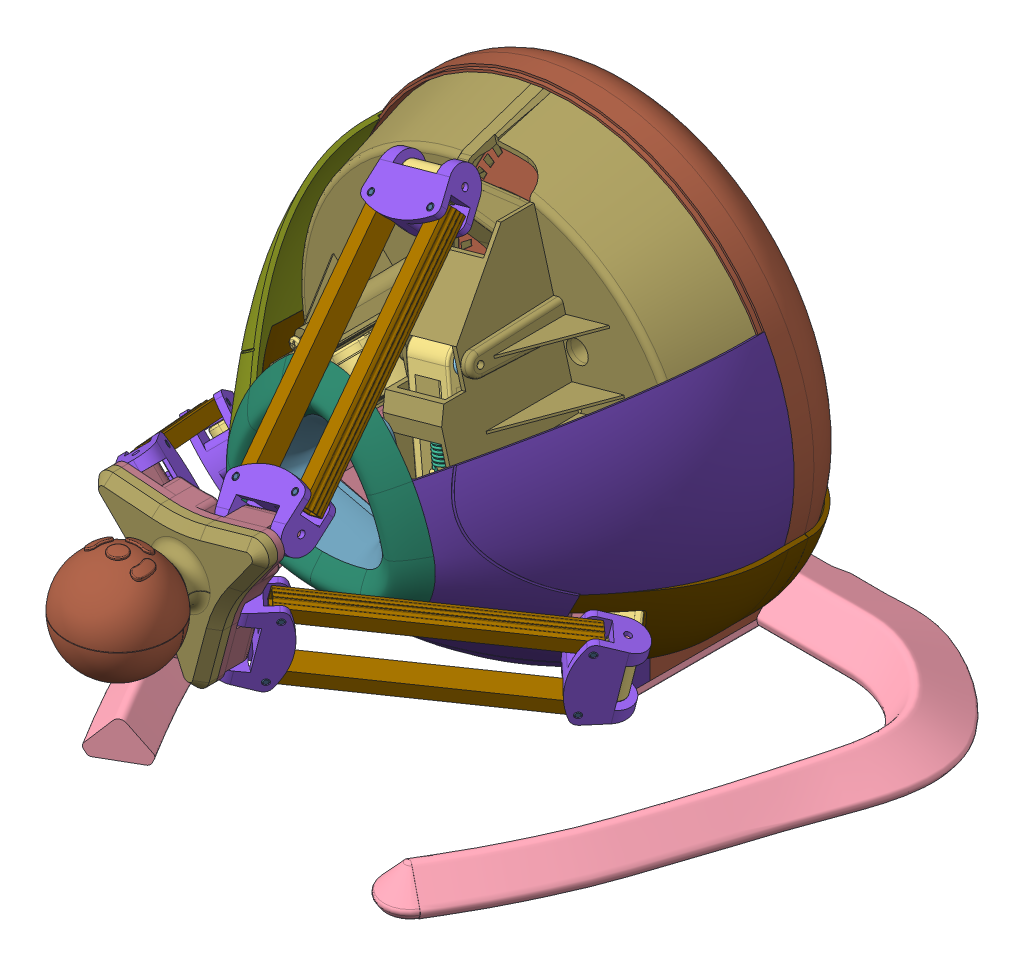
SolidWorks assembly 0_ROBOT_SET_corr, configuration Défaut. Lengths in mm.
Overall size (305.26 266.62 319.84).
141 component instances, 33 part files, 47 mates.
Components (placement in the parent):
- bati-1: bati [Défaut] at (0 -115.25 -99.3181) size (305.26 272.51 243.47)
  - MOTEUR-1: MOTEUR [Défaut] at (0.3122 36.9309 38.5) x (-0.700162 -0.713984 0) z (0 0 -1) size (38 68 38)
  - FIXATION MOTEUR-1: FIXATION MOTEUR [Défaut] at (-16.4664 53.3847 38.5) x (-0.700162 -0.713984 0) z (0.713984 -0.700162 0) size (53.2 19.6 6)
  - FIXATION MOTEUR-2: FIXATION MOTEUR [Défaut] at (-38.9569 75.4398 38.5) x (-0.700162 -0.713984 0) z (0.713984 -0.700162 0) size (53.2 19.6 6)
  - Vis à tôle tête cylindrique cruciforme H 2,9x13 - C-1: Vis à tôle tête cylindrique cruciforme H 2,9x13 - C [Réaliste] at (-32.9202 36.6061 36.1) x (0 0 1) z (0.023398 -0.999726 0) size (14.76 5.6 5.6)
  - Vis à tôle tête cylindrique cruciforme H 2,9x13 - C-2: Vis à tôle tête cylindrique cruciforme H 2,9x13 - C [Réaliste] at (-55.4107 58.6612 36.1) x (0 0 1) z (0.704809 -0.709397 0) size (14.76 5.6 5.6)
  - Vis à tôle tête cylindrique cruciforme H 2,9x13 - C-3: Vis à tôle tête cylindrique cruciforme H 2,9x13 - C [Réaliste] at (-0.0126 70.1633 36.1) x (0 0 1) z (0.824881 -0.565307 0) size (14.76 5.6 5.6)
  - Vis à tôle tête cylindrique cruciforme H 2,9x13 - C-4: Vis à tôle tête cylindrique cruciforme H 2,9x13 - C [Réaliste] at (-22.5031 92.2184 36.1) x (0 0 1) z (0.309324 0.950957 0) size (14.76 5.6 5.6)
  - socle-1: socle [Défaut] at (0 -1.5 37.7) x (1 0 0) z (0 1 0) size (305.26 243.47 58.01)
  - vis CHC M4-30-1: vis CHC M4-30 [Défaut] at (9.875 31.2 14.05) x (-0.866025 0 0.5) z (0 -1 0) size (7 7 34)
  - vis CHC M4-30-2: vis CHC M4-30 [Défaut] at (-9.875 31.2 14.05) x (-0.866025 0 0.5) z (0 -1 0) size (7 7 34)
  - Rondelle M4-1: Rondelle M4 [Défaut] at (9.875 2 14.05) x (0.991496 0 -0.130134) z (-0.130134 0 -0.991496) size (9 0.8 9)
  - Rondelle M4-2: Rondelle M4 [Défaut] at (-9.875 1.2 14.05) x (0.991496 0 -0.130134) z (0.130134 0 0.991496) size (9 0.8 9)
  - CARTE HEXAGONALE-1: CARTE HEXAGONALE [Défaut] at (0 115.25 16.9) x (-0.956305 -0.292372 0) z (0 0 -1) size (138.56 120 30)
  - Vis à tôle tête cylindrique cruciforme H 2,9x13 - C-5: Vis à tôle tête cylindrique cruciforme H 2,9x13 - C [Réaliste] at (0 115.25 -1.8) x (0 0 1) z (1 0 0) size (14.76 5.6 5.6)
  - petite carte-1: petite carte [Défaut] at (-5.4923 106.1588 52.9) x (-0.224951 -0.97437 0) z (0 0 -1) size (34.7 16 10.5)
  - Vis à tôle tête cylindrique cruciforme H 2,9x8 - C-1: Vis à tôle tête cylindrique cruciforme H 2,9x8 - C [Réaliste] at (-6.6871 74.3113 49.1) x (0 0 1) z (-1 0 0) size (9.76 5.6 5.6)
  - Vis à tôle tête cylindrique cruciforme H 2,9x13 - C-7: Vis à tôle tête cylindrique cruciforme H 2,9x13 - C [Réaliste] at (13.5332 64.175 13.6) x (0 0 1) z (-1 0 0) size (14.76 5.6 5.6)
  - Vis à tôle tête cylindrique cruciforme H 2,9x8 - C-2: Vis à tôle tête cylindrique cruciforme H 2,9x8 - C [Réaliste] at (38.7975 129.9282 49.1) x (0 0 1) z (0.5 -0.866025 0) size (9.76 5.6 5.6)
  - Vis à tôle tête cylindrique cruciforme H 2,9x8 - C-3: Vis à tôle tête cylindrique cruciforme H 2,9x8 - C [Réaliste] at (-32.1104 141.5105 49.1) x (0 0 1) z (0.5 0.866025 0) size (9.76 5.6 5.6)
  - petite carte-2: petite carte [Défaut] at (10.6194 115.0391 52.9) x (0.956305 0.292372 0) z (0 0 -1) size (34.7 16 10.5)
  - petite carte-3: petite carte [Défaut] at (-5.1271 124.5521 52.9) x (-0.731354 0.681998 0) z (0 0 -1) size (34.7 16 10.5)
  - Vis à tôle tête cylindrique cruciforme H 2,9x13 - C-8: Vis à tôle tête cylindrique cruciforme H 2,9x13 - C [Réaliste] at (31.1975 107.2775 36.1) x (0 0 1) z (-0.978215 -0.207596 0) size (14.76 5.6 5.6)
  - Vis à tôle tête cylindrique cruciforme H 2,9x13 - C-9: Vis à tôle tête cylindrique cruciforme H 2,9x13 - C [Réaliste] at (-8.6944 146.2541 36.1) x (0 0 1) z (0.668891 -0.74336 0) size (14.76 5.6 5.6)
  - Vis à tôle tête cylindrique cruciforme H 2,9x13 - C-10: Vis à tôle tête cylindrique cruciforme H 2,9x13 - C [Réaliste] at (39.0525 137.7824 36.1) x (0 0 1) z (0.07713 0.997021 0) size (14.76 5.6 5.6)
  - Vis à tôle tête cylindrique cruciforme H 2,9x13 - C-11: Vis à tôle tête cylindrique cruciforme H 2,9x13 - C [Réaliste] at (-39.0399 137.8043 36.1) x (0 0 1) z (-0.90201 -0.431714 0) size (14.76 5.6 5.6)
  - Vis à tôle tête cylindrique cruciforme H 2,9x13 - C-12: Vis à tôle tête cylindrique cruciforme H 2,9x13 - C [Réaliste] at (76.7127 95.5573 36.1) x (0 0 1) z (0.261951 0.965081 0) size (14.76 5.6 5.6)
  - Vis à tôle tête cylindrique cruciforme H 2,9x13 - C-13: Vis à tôle tête cylindrique cruciforme H 2,9x13 - C [Réaliste] at (-21.302 191.5315 36.1) x (0 0 1) z (-0.96676 -0.255684 0) size (14.76 5.6 5.6)
  - Vis à tôle tête cylindrique cruciforme H 2,9x13 - C-14: Vis à tôle tête cylindrique cruciforme H 2,9x13 - C [Réaliste] at (84.5678 126.0622 36.1) x (0 0 1) z (0.854089 0.520126 0) size (14.76 5.6 5.6)
  - Vis à tôle tête cylindrique cruciforme H 2,9x13 - C-15: Vis à tôle tête cylindrique cruciforme H 2,9x13 - C [Réaliste] at (-51.6475 183.0817 36.1) x (0 0 1) z (-0.877487 0.4796 0) size (14.76 5.6 5.6)
  - MOTEUR-2: MOTEUR [Défaut] at (67.6702 154.6799 38.5) x (0.968409 -0.249366 0) z (0 0 -1) size (38 68 38)
  - MOTEUR-3: MOTEUR [Défaut] at (-67.9825 154.1392 38.5) x (-0.268247 0.96335 0) z (0 0 -1) size (38 68 38)
  - FIXATION MOTEUR-3: FIXATION MOTEUR [Défaut] at (53.9551 101.4174 38.5) x (0.968409 -0.249366 0) z (0.249366 0.968409 0) size (53.2 19.6 6)
  - FIXATION MOTEUR-4: FIXATION MOTEUR [Défaut] at (-14.9982 168.8928 38.5) x (-0.268247 0.96335 0) z (-0.96335 -0.268247 0) size (53.2 19.6 6)
  - Vis à tôle tête cylindrique cruciforme H 2,9x13 - C-16: Vis à tôle tête cylindrique cruciforme H 2,9x13 - C [Réaliste] at (37.4657 152.5076 13.6) x (0 0 1) z (0.5 -0.866025 0) size (14.76 5.6 5.6)
  - Vis à tôle tête cylindrique cruciforme H 2,9x13 - C-17: Vis à tôle tête cylindrique cruciforme H 2,9x13 - C [Réaliste] at (-50.9989 129.0674 13.6) x (0 0 1) z (0.5 0.866025 0) size (14.76 5.6 5.6)
  - plaque fixation-1: plaque fixation [Défaut] at origin size (50 130.5 32.4)
  - CARTER ARRIERE-1: CARTER ARRIERE [Défaut] x (-1 0 0) z (0 0 -1) size (201 215.75 63.51)
  - carter transparant-5: carter transparant [Défaut] at (53.7597 64.2778 0) x (0.999684 -0.02513 0) z (0 0 1) size (254.04 231.73 115.3)
    - carter transparant-1: carter transparant [Défaut] at (-154.833 107.2301 0) x (-0.5 -0.866025 0) z (0 0 1) size (168.6 94.54 100.3)
    - carter transparant2-1: carter transparant2 [Défaut] at (-55.0236 -65.6449 0) size (168.6 126.77 115.3)
    - carter transparant-2: carter transparant [Défaut] at (44.7858 107.2301 0) x (-0.5 0.866025 0) z (0 0 1) size (168.6 94.54 100.3)
  - Vis à tôle tête cylindrique cruciforme H 2,9x13 - C-18: Vis à tôle tête cylindrique cruciforme H 2,9x13 - C [Réaliste] at (78.1771 88.895 19.2) x (0 0 1) z (-0.823437 0.567408 0) size (14.76 5.6 5.6)
  - Vis à tôle tête cylindrique cruciforme H 2,9x13 - C-19: Vis à tôle tête cylindrique cruciforme H 2,9x13 - C [Réaliste] at (56.5905 55.2187 19.2) x (0 0 1) z (-1 0 0) size (14.76 5.6 5.6)
  - Vis à tôle tête cylindrique cruciforme H 2,9x13 - C-20: Vis à tôle tête cylindrique cruciforme H 2,9x13 - C [Réaliste] at (23.6934 194.2745 19.2) x (0 0 1) z (0.5 -0.866025 0) size (14.76 5.6 5.6)
  - Vis à tôle tête cylindrique cruciforme H 2,9x13 - C-21: Vis à tôle tête cylindrique cruciforme H 2,9x13 - C [Réaliste] at (-80.2839 96.2568 19.2) x (0 0 1) z (0.5 0.866025 0) size (14.76 5.6 5.6)
  - Vis à tôle tête cylindrique cruciforme H 2,9x13 - C-22: Vis à tôle tête cylindrique cruciforme H 2,9x13 - C [Réaliste] at (-16.2645 196.1309 19.2) x (0 0 1) z (-0.079672 -0.996821 0) size (14.76 5.6 5.6)
  - Vis à tôle tête cylindrique cruciforme H 2,9x13 - C-23: Vis à tôle tête cylindrique cruciforme H 2,9x13 - C [Réaliste] at (-61.9127 60.7241 19.2) x (0 0 1) z (0.903108 0.429413 0) size (14.76 5.6 5.6)
  - carter avant-1: carter avant [Défaut] at (17.1026 113.9098 24) size (270.48 238.53 119.64)
    - carter avant01-1: carter avant01 [Défaut] at (-17.1026 -113.9098 0) size (187.24 89.78 114.01) (hidden)
    - carter avant1-1: carter avant1 [Défaut] at (-17.1026 -113.9098 0) size (64.62 62.88 20.8)
    - CARTER NEZ-1: CARTER NEZ [Défaut] x (-1 0 0) z (0 1 0) size (94.64 9.63 92.67)
    - carter avant02-1: carter avant02 [Défaut] at (82.7068 58.9652 0) x (-0.5 0.866025 0) z (0 0 1) size (193.15 89.78 114.01)
    - carter avant03-1: carter avant03 [Défaut] at (-116.9121 58.9652 0) x (-0.5 -0.866025 0) z (0 0 1) size (191.25 89.78 114.01)
    - Vis à tôle tête cylindrique cruciforme H 2,9x13 - C-1: Vis à tôle tête cylindrique cruciforme H 2,9x13 - C [Réaliste] at (-32.0102 -41.9914 97) x (0 0 -1) z (1 0 0) size (14.76 5.6 5.6)
    - Vis à tôle tête cylindrique cruciforme H 2,9x13 - C-2: Vis à tôle tête cylindrique cruciforme H 2,9x13 - C [Réaliste] at (-47.1751 35.9163 97) x (0 0 -1) z (1 0 0) size (14.76 5.6 5.6)
    - Vis à tôle tête cylindrique cruciforme H 2,9x13 - C-3: Vis à tôle tête cylindrique cruciforme H 2,9x13 - C [Réaliste] at (27.8774 10.0956 97) x (0 0 -1) z (1 0 0) size (14.76 5.6 5.6)
  - FIXATION MOTEUR-5: FIXATION MOTEUR [Défaut] at (61.8101 131.9223 38.5) x (0.968409 -0.249366 0) z (0.249366 0.968409 0) size (53.2 19.6 6)
  - FIXATION MOTEUR-6: FIXATION MOTEUR [Défaut] at (-45.3437 160.443 38.5) x (-0.268247 0.96335 0) z (-0.96335 -0.268247 0) size (53.2 19.6 6)
  - PLAQUE NOM-1: PLAQUE NOM [Défaut] at (0 0 138) size (62.75 60.78 0.1) (hidden)
  - CACHE-1: CACHE [Défaut] at (0 0 24) size (77.2 40.92 103.91) (hidden)
  - CACHE-2: CACHE [Défaut] at (99.8094 172.875 24) x (-0.5 0.866025 0) z (0 0 1) size (77.2 40.92 103.91)
  - CACHE-3: CACHE [Défaut] at (-99.8094 172.875 24) x (-0.5 -0.866025 0) z (0 0 1) size (77.2 40.92 103.91)
- ROTOR-1: ROTOR [Défaut] at (-39.1783 46.9097 -60.8181) x (-0.96335 -0.268247 0) z (-0.263807 0.947405 -0.181189) size (89.6 91.37 91.37)
  - ROTOR-1: ROTOR [Défaut] at (30.9 0 0) x (0 0.28167 0.959511) z (0 -0.959511 0.28167) size (27 85 27)
  - ROUE CODEUSE-1: ROUE CODEUSE [Défaut] at (-36.4 0 0) x (0 0.892316 -0.451411) z (0 0.451411 0.892316) size (68 22.3 68)
- bras-6: bras [Défaut] at (-132.6853 -42.6289 -14.2354) x (-0.96335 -0.268247 0) z (0.04356 -0.156434 -0.986727) size (30 123.88 64.5)
  - bras-1: bras [Défaut] at (-166.5919 39.8256 -20.981) x (0 0 1) z (-1 0 0) size (64.5 123.88 20.1)
  - AXE BRAS-1: AXE BRAS [Défaut] at (-166.5919 39.8256 -20.981) x (0 0 -1) z (1 0 0) size (3 3 30)
  - palier bras-1: palier bras [Défaut] at origin size (5 10 10)
  - palier bras-2: palier bras [Défaut] at (-333.1838 5.2271 7.8152) x (-1 0 0) z (0 -0.924225 -0.381849) size (5 10 10)
  - Ressort cable-1: Ressort cable [Défaut] at (-166.5919 17.1829 -24.981) x (1 0 0) z (0 -1 0) size (9.03 7.82 23.53)
  - FIXATION CABLE-1: FIXATION CABLE [Défaut] at (-172.5919 90.5863 3.4188) x (1 0 0) z (0 0.85 0.526783) size (4 4 0.2)
- joint-10: joint [Défaut] at (-150.363 16.9955 177.0225) x (-0.96335 -0.268247 0) z (0.215517 -0.773981 0.595404) size (37.18 21.16 28.81)
  - joint-1: joint [Défaut] at (-167.6277 128.0999 -150.9355) x (1 0 0) z (0 -0.97714 -0.212597) size (37.18 26 16)
  - AXE BRAS-1: AXE BRAS [Défaut] at (-167.6277 126.3991 -143.1184) x (0 0 1) z (-1 0 0) size (3 3 30)
- BIELLE PARALLELOGRAMME-10: BIELLE PARALLELOGRAMME [Défaut] at (181.3498 63.6696 78.3777) x (0.967438 0.252419 0.018681) z (0.152669 -0.640809 0.752367) size (7.16 16 109)
  - BIELLE PARALLELOGRAMME-1: BIELLE PARALLELOGRAMME [Défaut] at (-178.1288 5 -54.5) x (0 -1 0) z (0 0 -1) size (10 7.16 109)
  - AXE BIELLE-1: AXE BIELLE [Défaut] at (-181.1288 5 -105.75) x (0.623444 0 0.781868) z (0 1 0) size (3 3 16)
  - AXE BIELLE-2: AXE BIELLE [Défaut] at (-181.1288 5 -3.25) x (0.623444 0 0.781868) z (0 1 0) size (3 3 16)
- BIELLE PARALLELOGRAMME-11: BIELLE PARALLELOGRAMME [Défaut] at (-144.1569 -13.01 78.1952) x (-0.967438 -0.252419 -0.018681) z (0.152669 -0.640809 0.752367) size (7.16 16 109)
  - BIELLE PARALLELOGRAMME-1: BIELLE PARALLELOGRAMME [Défaut] at (-178.1288 5 -54.5) x (0 -1 0) z (0 0 -1) size (10 7.16 109)
  - AXE BIELLE-1: AXE BIELLE [Défaut] at (-181.1288 5 -105.75) x (0.623444 0 0.781868) z (0 1 0) size (3 3 16)
  - AXE BIELLE-2: AXE BIELLE [Défaut] at (-181.1288 5 -3.25) x (0.623444 0 0.781868) z (0 1 0) size (3 3 16)
- joint-11: joint [Défaut] at (-152.0533 13.5809 -102.4577) x (-0.96335 -0.268247 0) z (-0.215517 0.773981 -0.595404) size (37.18 21.16 28.81)
  - joint-1: joint [Défaut] at (-167.6277 128.0999 -150.9355) x (1 0 0) z (0 -0.97714 -0.212597) size (37.18 26 16)
  - AXE BRAS-1: AXE BRAS [Défaut] at (-167.6277 126.3991 -143.1184) x (0 0 1) z (-1 0 0) size (3 3 30)
- ROTOR-2: ROTOR [Défaut] at (59.9648 9.506 -60.8181) x (0.249366 0.968409 0) z (0.867368 -0.223348 0.444734) size (89.6 91.37 91.37)
  - ROTOR-1: ROTOR [Défaut] at (30.9 0 0) x (0 0.28167 0.959511) z (0 -0.959511 0.28167) size (27 85 27)
  - ROUE CODEUSE-1: ROUE CODEUSE [Défaut] at (-36.4 0 0) x (0 0.892316 -0.451411) z (0 0.451411 0.892316) size (68 22.3 68)
- bras-5: bras [Défaut] at (29.4658 136.2127 -14.3614) x (0.249366 0.968409 0) z (-0.154435 0.039767 -0.987202) size (30 123.88 64.5)
  - bras-1: bras [Défaut] at (-166.5919 39.8256 -20.981) x (0 0 1) z (-1 0 0) size (64.5 123.88 20.1)
  - AXE BRAS-1: AXE BRAS [Défaut] at (-166.5919 39.8256 -20.981) x (0 0 -1) z (1 0 0) size (3 3 30)
  - palier bras-1: palier bras [Défaut] at origin size (5 10 10)
  - palier bras-2: palier bras [Défaut] at (-333.1838 5.2271 7.8152) x (-1 0 0) z (0 -0.924225 -0.381849) size (5 10 10)
  - Ressort cable-1: Ressort cable [Défaut] at (-166.5919 17.1829 -24.981) x (1 0 0) z (0 -1 0) size (9.03 7.82 23.53)
  - FIXATION CABLE-1: FIXATION CABLE [Défaut] at (-172.5919 90.5863 3.4188) x (1 0 0) z (0 0.85 0.526783) size (4 4 0.2)
- joint-12: joint [Défaut] at (89.5321 121.8152 177.1099) x (0.249366 0.968409 0) z (-0.779305 0.200672 0.593645) size (37.18 21.16 28.81)
  - joint-1: joint [Défaut] at (-167.6277 128.0999 -150.9355) x (1 0 0) z (0 -0.97714 -0.212597) size (37.18 26 16)
  - AXE BRAS-1: AXE BRAS [Défaut] at (-167.6277 126.3991 -143.1184) x (0 0 1) z (-1 0 0) size (3 3 30)
- BIELLE PARALLELOGRAMME-9: BIELLE PARALLELOGRAMME [Défaut] at (40.919 -211.3723 2.7018) x (-0.263213 -0.964599 0.01634) z (0.633694 -0.18564 -0.750979) size (7.16 16 109)
  - BIELLE PARALLELOGRAMME-1: BIELLE PARALLELOGRAMME [Défaut] at (-178.1288 5 -54.5) x (0 -1 0) z (0 0 -1) size (10 7.16 109)
  - AXE BIELLE-1: AXE BIELLE [Défaut] at (-181.1288 5 -105.75) x (0.623444 0 0.781868) z (0 1 0) size (3 3 16)
  - AXE BIELLE-2: AXE BIELLE [Défaut] at (-181.1288 5 -3.25) x (0.623444 0 0.781868) z (0 1 0) size (3 3 16)
- BIELLE PARALLELOGRAMME-12: BIELLE PARALLELOGRAMME [Défaut] at (60.2151 131.1803 78.6391) x (0.263213 0.964599 -0.01634) z (-0.633694 0.18564 0.750979) size (7.16 16 109)
  - BIELLE PARALLELOGRAMME-1: BIELLE PARALLELOGRAMME [Défaut] at (-178.1288 5 -54.5) x (0 -1 0) z (0 0 -1) size (10 7.16 109)
  - AXE BIELLE-1: AXE BIELLE [Défaut] at (-181.1288 5 -105.75) x (0.623444 0 0.781868) z (0 1 0) size (3 3 16)
  - AXE BIELLE-2: AXE BIELLE [Défaut] at (-181.1288 5 -3.25) x (0.623444 0 0.781868) z (0 1 0) size (3 3 16)
- joint-9: joint [Défaut] at (87.9291 124.5304 -102.3703) x (0.249366 0.968409 0) z (0.779305 -0.200672 -0.593645) size (37.18 21.16 28.81)
  - joint-1: joint [Défaut] at (-167.6277 128.0999 -150.9355) x (1 0 0) z (0 -0.97714 -0.212597) size (37.18 26 16)
  - AXE BRAS-1: AXE BRAS [Défaut] at (-167.6277 126.3991 -143.1184) x (0 0 1) z (-1 0 0) size (3 3 30)
- ROTOR-3: ROTOR [Défaut] at (-21.7499 -56.6842 -60.8181) x (0.713984 -0.700162 0) z (0.616556 0.628727 0.473879) size (89.6 91.37 91.37)
  - ROTOR-1: ROTOR [Défaut] at (30.9 0 0) x (0 0.28167 0.959511) z (0 -0.959511 0.28167) size (27 85 27)
  - ROUE CODEUSE-1: ROUE CODEUSE [Défaut] at (-36.4 0 0) x (0 0.892316 -0.451411) z (0 0.451411 0.892316) size (68 22.3 68)
- bras-2: bras [Défaut] at (103.2171 -93.6385 -14.4192) x (0.713984 -0.700162 0) z (0.11072 0.112906 -0.987418) size (30 123.88 64.5)
  - bras-1: bras [Défaut] at (-166.5919 39.8256 -20.981) x (0 0 1) z (-1 0 0) size (64.5 123.88 20.1)
  - AXE BRAS-1: AXE BRAS [Défaut] at (-166.5919 39.8256 -20.981) x (0 0 -1) z (1 0 0) size (3 3 30)
  - palier bras-1: palier bras [Défaut] at origin size (5 10 10)
  - palier bras-2: palier bras [Défaut] at (-333.1838 5.2271 7.8152) x (-1 0 0) z (0 -0.924225 -0.381849) size (5 10 10)
  - Ressort cable-1: Ressort cable [Défaut] at (-166.5919 17.1829 -24.981) x (1 0 0) z (0 -1 0) size (9.03 7.82 23.53)
  - FIXATION CABLE-1: FIXATION CABLE [Défaut] at (-172.5919 90.5863 3.4188) x (1 0 0) z (0 0.85 0.526783) size (4 4 0.2)
- joint-4: joint [Défaut] at (60.8403 -138.3312 177.1532) x (0.713984 -0.700162 0) z (0.563822 0.574952 0.592904) size (37.18 21.16 28.81)
  - joint-1: joint [Défaut] at (-167.6277 128.0999 -150.9355) x (1 0 0) z (0 -0.97714 -0.212597) size (37.18 26 16)
  - AXE BRAS-1: AXE BRAS [Défaut] at (-167.6277 126.3991 -143.1184) x (0 0 1) z (-1 0 0) size (3 3 30)
- BIELLE PARALLELOGRAMME-3: BIELLE PARALLELOGRAMME [Défaut] at (36.4709 -162.2811 -10.0756) x (0.702583 -0.71137 -0.018156) z (-0.479813 -0.454737 -0.750329) size (7.16 16 109)
  - BIELLE PARALLELOGRAMME-1: BIELLE PARALLELOGRAMME [Défaut] at (-178.1288 5 -54.5) x (0 -1 0) z (0 0 -1) size (10 7.16 109)
  - AXE BIELLE-1: AXE BIELLE [Défaut] at (-181.1288 5 -105.75) x (0.623444 0 0.781868) z (0 1 0) size (3 3 16)
  - AXE BIELLE-2: AXE BIELLE [Défaut] at (-181.1288 5 -3.25) x (0.623444 0 0.781868) z (0 1 0) size (3 3 16)
- BIELLE PARALLELOGRAMME-4: BIELLE PARALLELOGRAMME [Défaut] at (-203.3086 70.4548 3.1096) x (-0.702583 0.71137 0.018156) z (-0.479813 -0.454737 -0.750329) size (7.16 16 109)
  - BIELLE PARALLELOGRAMME-1: BIELLE PARALLELOGRAMME [Défaut] at (-178.1288 5 -54.5) x (0 -1 0) z (0 0 -1) size (10 7.16 109)
  - AXE BIELLE-1: AXE BIELLE [Défaut] at (-181.1288 5 -105.75) x (0.623444 0 0.781868) z (0 1 0) size (3 3 16)
  - AXE BIELLE-2: AXE BIELLE [Défaut] at (-181.1288 5 -3.25) x (0.623444 0 0.781868) z (0 1 0) size (3 3 16)
- joint-3: joint [Défaut] at (63.9887 -138.6619 -102.3333) x (0.713984 -0.700162 0) z (-0.563822 -0.574952 -0.592904) size (37.18 21.16 28.81)
  - joint-1: joint [Défaut] at (-167.6277 128.0999 -150.9355) x (1 0 0) z (0 -0.97714 -0.212597) size (37.18 26 16)
  - AXE BRAS-1: AXE BRAS [Défaut] at (-167.6277 126.3991 -143.1184) x (0 0 1) z (-1 0 0) size (3 3 30)
- poignee-1: poignee [Défaut] at (46.3334 -98.96 -94.3816) x (0.999684 -0.02513 0) z (0 0 1) size (91.69 95.36 94.16)
  - manette2-1: manette2 [Défaut] at (-49.9574 99.5142 190.1896) x (-0.954964 0.29672 0) z (0 0 1) size (46.3 47.3 60.42)
  - manette-1: manette [Default] at (-75.5797 129.3549 187.9639) x (-0.954964 0.29672 0) z (0 0 1) size (71.94 77.5 39.3)
    - manette1-1: manette1 [Défaut] at (-33.3227 20.8941 2.2257) size (71.94 77.5 39.3)
  - EFFECTEUR-1: EFFECTEUR [Défaut] at origin size (85.21 85.35 36.25)
    - BASE-1: BASE [Défaut] at (-48.8094 97.9143 187.1896) x (0.990623 -0.136626 0) z (0 0 1) size (75.58 75.74 36.25)
Mates (geometry in assembly coordinates):
- Coaxiale34: concentric: cylinder of joint-3/joint-1 through (-38.4703 16.2646 70.5778) axis (-0.525506 -0.53588 0.660815) radius 1.5; cylinder of BIELLE PARALLELOGRAMME-3/AXE BIELLE-1 through (-46.8784 7.6905 81.1508) axis (0.525506 0.53588 -0.660815) radius 1.5
- Coïncidente34: coincident: plane of joint-3/joint-1 through (-23.772 11.2576 90.3124) normal (0.525506 0.53588 -0.660815); plane of BIELLE PARALLELOGRAMME-3/AXE BIELLE-1 through (-42.6743 11.9775 75.8643) normal (-0.525506 -0.53588 0.660815)
- Coaxiale37: concentric: cylinder of bras-2/bras-1 through (-94.2044 -42.7415 -9.4881) axis (0.713984 -0.700162 0) radius 1.5; cylinder of joint-4/AXE BRAS-1 through (-97.7743 -39.2407 -9.4881) axis (0.713984 -0.700162 0) radius 1.5
- Coïncidente37: coincident: plane of bras-2/bras-1 through (-45.5834 -7.4431 0) normal (-0.713984 0.700162 0); plane of joint-4/joint-1
- Coaxiale38: concentric: cylinder of BIELLE PARALLELOGRAMME-3/AXE BIELLE-2 through (-96.0592 -38.92 4.2421) axis (0.525506 0.53588 -0.660815) radius 1.5; cylinder of joint-4/joint-1 through (-96.0592 -38.92 4.2421) axis (0.525506 0.53588 -0.660815) radius 1.5
- Coïncidente38: coincident: plane of BIELLE PARALLELOGRAMME-3/BIELLE PARALLELOGRAMME-1; plane of joint-4/joint-1 through (-90.766 -53.5176 -15.4925) normal (-0.525506 -0.53588 0.660815)
- Coaxiale39: concentric: cylinder of joint-3/joint-1 through (-18.4787 -3.34 70.5778) axis (-0.525506 -0.53588 0.660815) radius 1.5; cylinder of BIELLE PARALLELOGRAMME-4/AXE BIELLE-1 through (-18.4787 -3.34 70.5778) axis (-0.525506 -0.53588 0.660815) radius 1.5
- Coaxiale40: concentric: cylinder of BIELLE PARALLELOGRAMME-4/AXE BIELLE-2 through (-67.6596 -49.9505 -6.3309) axis (-0.525506 -0.53588 0.660815) radius 1.5; cylinder of joint-4/joint-1 through (-76.0677 -58.5246 4.2421) axis (0.525506 0.53588 -0.660815) radius 1.5
- Coïncidente39: coincident: plane of BIELLE PARALLELOGRAMME-4/BIELLE PARALLELOGRAMME-1; plane of joint-4/joint-1 through (-90.766 -53.5176 -15.4925) normal (-0.525506 -0.53588 0.660815)
- Coaxiale52: concentric: cylinder of bras-5/bras-1 through (84.1049 -60.2095 -9.5684) axis (0.249366 0.968409 0) radius 1.5; cylinder of joint-12/AXE BRAS-1 through (82.8581 -65.0515 -9.5684) axis (0.249366 0.968409 0) radius 1.5
- Coïncidente50: coincident: plane of bras-5/bras-1 through (29.2376 -35.7549 0) normal (-0.249366 -0.968409 0); plane of joint-12/joint-1
- Coaxiale53: concentric: cylinder of BIELLE PARALLELOGRAMME-12/AXE BIELLE-1 through (70.0962 -60.7327 -6.3989) axis (0.727427 -0.187313 0.660124) radius 1.5; cylinder of joint-12/joint-1 through (81.735 -63.7297 4.1631) axis (-0.727427 0.187313 -0.660124) radius 1.5
- Coïncidente51: coincident: plane of BIELLE PARALLELOGRAMME-12/BIELLE PARALLELOGRAMME-1 through (82.4019 -60.8773 -0.307) normal (0.727427 -0.187313 0.660124); plane of joint-12/joint-1 through (101.4665 -54.3539 -19.4642) normal (-0.727427 0.187313 -0.660124)
- Coaxiale54: concentric: cylinder of BIELLE PARALLELOGRAMME-9/AXE BIELLE-2 through (77.0785 -33.6173 -6.3989) axis (0.727427 -0.187313 0.660124) radius 1.5; cylinder of joint-12/joint-1 through (88.7173 -36.6143 4.1631) axis (-0.727427 0.187313 -0.660124) radius 1.5
- Coïncidente52: coincident: plane of BIELLE PARALLELOGRAMME-9/BIELLE PARALLELOGRAMME-1 through (18.7322 -19.3147 81.6478) normal (0.727427 -0.187313 0.660124); plane of joint-12/joint-1 through (101.4665 -54.3539 -19.4642) normal (-0.727427 0.187313 -0.660124)
- Coaxiale57: concentric: cylinder of BIELLE PARALLELOGRAMME-12/AXE BIELLE-2 through (5.1426 -41.7046 70.5765) axis (0.727427 -0.187313 0.660124) radius 1.5; cylinder of joint-9/joint-1 through (5.1426 -41.7046 70.5765) axis (0.727427 -0.187313 0.660124) radius 1.5
- Coïncidente55: coincident: plane of BIELLE PARALLELOGRAMME-12/BIELLE PARALLELOGRAMME-1 through (75.1276 -59.0042 -6.9082) normal (-0.727427 0.187313 -0.660124); plane of joint-9/joint-1 through (-7.6066 -23.965 94.2038) normal (0.727427 -0.187313 0.660124)
- Coaxiale59: concentric: cylinder of BIELLE PARALLELOGRAMME-9/AXE BIELLE-1 through (12.1248 -14.5892 70.5765) axis (0.727427 -0.187313 0.660124) radius 1.5; cylinder of joint-9/joint-1 through (12.1248 -14.5892 70.5765) axis (0.727427 -0.187313 0.660124) radius 1.5
- Coaxiale60: concentric: cylinder of bras-6/bras-1 through (10.0981 102.9142 -9.7432) axis (-0.96335 -0.268247 0) radius 1.5; cylinder of joint-10/AXE BRAS-1 through (14.9149 104.2554 -9.7432) axis (-0.96335 -0.268247 0) radius 1.5
- Coïncidente57: coincident: plane of bras-6/bras-1 through (16.3458 43.1979 0) normal (0.96335 0.268247 0); plane of joint-10/joint-1
- Coaxiale61: concentric: cylinder of BIELLE PARALLELOGRAMME-11/AXE BIELLE-1 through (17.5537 91.0507 -6.5442) axis (-0.201883 0.725016 0.658479) radius 1.5; cylinder of joint-10/joint-1 through (14.3236 102.6509 3.9914) axis (0.201883 -0.725016 -0.658479) radius 1.5
- Coïncidente58: coincident: plane of BIELLE PARALLELOGRAMME-11/BIELLE PARALLELOGRAMME-1; plane of joint-10/joint-1
- Coaxiale62: concentric: cylinder of BIELLE PARALLELOGRAMME-11/AXE BIELLE-2 through (33.2022 25.3678 70.5734) axis (-0.201883 0.725016 0.658479) radius 1.5; cylinder of joint-11/joint-1 through (33.2022 25.3678 70.5734) axis (-0.201883 0.725016 0.658479) radius 1.5
- Coïncidente59: coincident: plane of BIELLE PARALLELOGRAMME-11/BIELLE PARALLELOGRAMME-1; plane of joint-11/joint-1
- Coaxiale63: concentric: cylinder of BIELLE PARALLELOGRAMME-10/AXE BIELLE-1 through (-12.6502 95.14 3.9914) axis (0.201883 -0.725016 -0.658479) radius 1.5; cylinder of joint-10/joint-1 through (-12.6502 95.14 3.9914) axis (0.201883 -0.725016 -0.658479) radius 1.5
- Coïncidente60: coincident: plane of BIELLE PARALLELOGRAMME-10/BIELLE PARALLELOGRAMME-1 through (-9.6384 95.8048 -0.3732) normal (-0.201883 0.725016 0.658479); plane of joint-10/joint-1 through (-3.648 115.0011 -19.6726) normal (0.201883 -0.725016 -0.658479)
- Coaxiale64: concentric: cylinder of BIELLE PARALLELOGRAMME-10/AXE BIELLE-2 through (2.9983 29.4571 81.1091) axis (0.201883 -0.725016 -0.658479) radius 1.5; cylinder of joint-11/joint-1 through (6.2284 17.8568 70.5734) axis (-0.201883 0.725016 0.658479) radius 1.5
- Coaxiale65: concentric: cylinder of bati-1/carter transparant-5/carter transparant2-1 through (7.8479 -118.8216 0) axis (0.249366 0.968409 0) radius 1.5; cylinder of bras-5/palier bras-2 through (33.1977 -20.376 0) axis (0.249366 0.968409 0) radius 3
- Coïncidente62: coincident: plane of bati-1/carter transparant-5/carter transparant2-1 through (66.6689 -57.2686 -39.4123) normal (0.249366 0.968409 0); plane of bras-5/palier bras-1 through (23.5018 -46.1531 0.4784) normal (-0.249366 -0.968409 0)
- Coïncidente63: coincident: plane of bati-1/carter transparant-5/carter transparant-2 through (16.2616 86.3712 -39.4123) normal (-0.96335 -0.268247 0); plane of bras-6/palier bras-1 through (28.2184 43.431 0.4872) normal (0.96335 0.268247 0)
- Coaxiale66: concentric: cylinder of bati-1/carter transparant-5/carter transparant-2 through (-50.2952 24.6415 0) axis (0.96335 0.268247 0) radius 1.5; cylinder of bras-6/palier bras-1 through (31.6444 47.4578 0) axis (0.96335 0.268247 0) radius 3
- Coaxiale67: concentric: cylinder of bati-1/carter transparant-5/carter transparant-1 through (-106.8264 52.6143 0) axis (0.713984 -0.700162 0) radius 1.5; cylinder of bras-2/palier bras-2 through (-34.245 -18.5621 0) axis (0.713984 -0.700162 0) radius 3
- Coïncidente64: coincident: plane of bati-1/carter transparant-5/carter transparant-1 through (-24.324 -2.1888 -82.4181) normal (-0.713984 0.700162 0); plane of bras-2/palier bras-2 through (-36.2736 -14.3743 -2.5566) normal (0.713984 -0.700162 0)
- Coaxiale73: concentric: cylinder of bati-1/MOTEUR-1 through (0.3122 -78.3192 -60.8181) axis (0.713984 -0.700162 0) radius 19; cylinder of ROTOR-3/ROTOR-1 through (0.3122 -78.3192 -60.8181) axis (0.713984 -0.700162 0) radius 1.6
- Distance1: distance = 2.6 mm: plane of bati-1/MOTEUR-1 through (-0.4239 -75.3564 -60.8181) normal (0.713984 -0.700162 0); plane of ROTOR-3/ROTOR-1 through (0.3122 -78.3192 -60.8181) normal (0.713984 -0.700162 0)
- Coaxiale74: concentric: cylinder of bati-1/MOTEUR-3 through (-67.9825 38.8891 -60.8181) axis (-0.96335 -0.268247 0) radius 19; cylinder of ROTOR-1/ROTOR-1 through (-68.9458 38.6209 -60.8181) axis (-0.96335 -0.268247 0) radius 1.6
- Distance2: distance = 3.6 mm: plane of ROTOR-1/ROTOR-1 through (-68.9458 38.6209 -60.8181) normal (-0.96335 -0.268247 0); plane of bati-1/MOTEUR-3 through (-65.0485 38.0452 -60.8181) normal (-0.96335 -0.268247 0)
- Coaxiale75: concentric: cylinder of bati-1/MOTEUR-2 through (67.6702 39.4299 -60.8181) axis (0.249366 0.968409 0) radius 19; cylinder of ROTOR-2/ROTOR-1 through (67.6702 39.4299 -60.8181) axis (0.249366 0.968409 0) radius 13.5
- Distance3: distance = 2.6 mm: plane of ROTOR-2/ROTOR-1 through (67.6702 39.4299 -60.8181) normal (0.249366 0.968409 0); plane of bati-1/MOTEUR-2 through (65.4724 37.311 -60.8181) normal (0.249366 0.968409 0)
- Coaxiale76: concentric: cylinder of joint-3/AXE BRAS-1 through (-38.1832 17.9856 84.308) axis (0.713984 -0.700162 0) radius 1.5; cylinder of poignee-1/EFFECTEUR-1/BASE-1 through (-48.2444 27.852 84.308) axis (0.713984 -0.700162 0) radius 1.5
- Coïncidente73: coincident: plane of joint-3/joint-1 through (-35.9117 13.5178 97.6241) normal (0.713984 -0.700162 0); plane of poignee-1/EFFECTEUR-1/BASE-1 through (-38.2926 11.0899 84.308) normal (-0.713984 0.700162 0)
- Coaxiale77: concentric: cylinder of poignee-1/EFFECTEUR-1/BASE-1 through (38.2859 25.3435 84.308) axis (-0.96335 -0.268247 0) radius 1.5; cylinder of joint-11/AXE BRAS-1 through (34.5377 24.2998 84.308) axis (-0.96335 -0.268247 0) radius 1.5
- Coïncidente74: coincident: plane of poignee-1/EFFECTEUR-1/BASE-1 through (28.6205 27.8423 84.308) normal (0.96335 0.268247 0); plane of joint-11/joint-1 through (29.5216 24.6063 97.6191) normal (-0.96335 -0.268247 0)
- Coaxiale78: concentric: cylinder of poignee-1/EFFECTEUR-1/BASE-1 through (1.9961 -48.2409 84.308) axis (0.249366 0.968409 0) radius 1.5; cylinder of joint-9/AXE BRAS-1 through (3.5208 -42.3197 84.308) axis (0.249366 0.968409 0) radius 1.5
- Coïncidente75: coincident: plane of poignee-1/EFFECTEUR-1/BASE-1 through (14.6594 -19.1142 84.308) normal (0.249366 0.968409 0); plane of joint-9/joint-1 through (11.3781 -18.2692 97.6226) normal (-0.249366 -0.968409 0)
- Angle4: planar angle = 1.727876 rad anti-aligned: unknown of bras-6/palier bras-1
- Coïncidente82: coincident: line of ? through (0 0 154.8075) axis (0 0 1)
